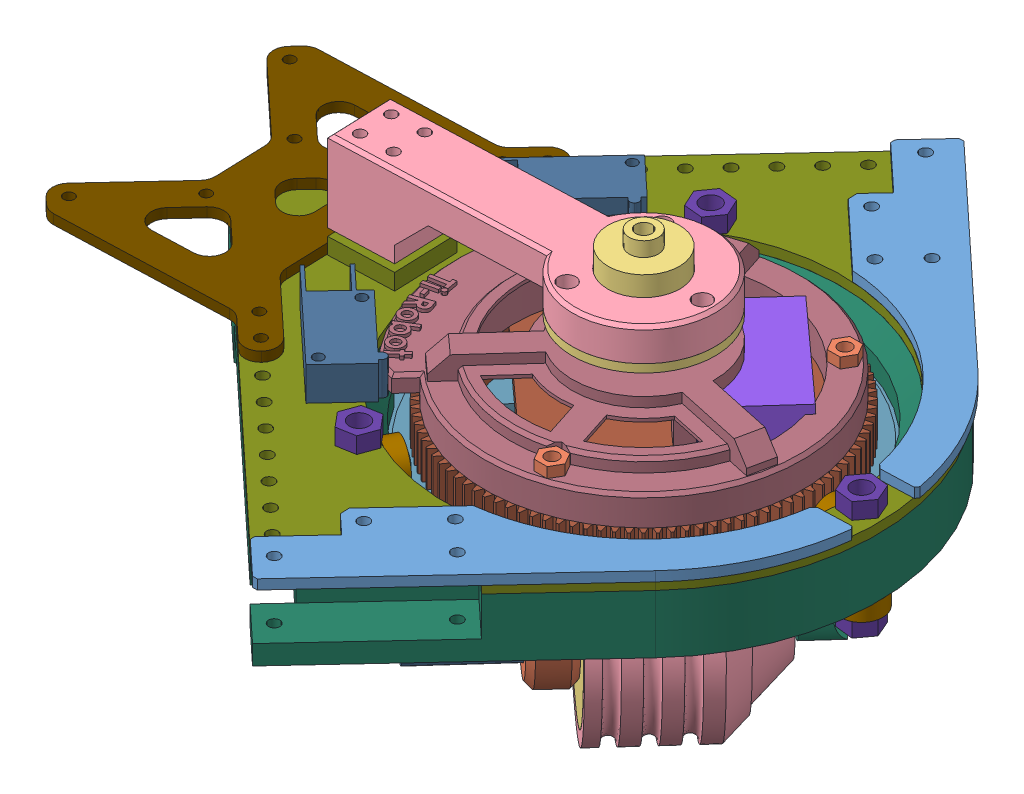
SolidWorks assembly swerve_unit, configuration ﾃﾞﾌｫﾙﾄ. Lengths in mm.
Overall size (282.67 132.43 227.55).
39 component instances, 23 part files, 96 mates.
Components (placement in the parent):
- M3508^swerve_unit-1: M3508^swerve_unit [ﾃﾞﾌｫﾙﾄ] at (107.8783 -47.57 102.4913) x (0 1 0) z (0.742238 0 0.670137) size (42 98.4 42) (virtual)
- motor_base^swerve_unit-1: motor_base^swerve_unit [ﾃﾞﾌｫﾙﾄ] at (107.8783 -47.57 102.4913) x (0 -1 0) z (0.670137 0 -0.742238) size (52 54 43) (virtual)
- bear_1^swerve_unit-1: bear_1^swerve_unit [ﾃﾞﾌｫﾙﾄ] at (129.3399 -43.5484 159.5919) x (0.723464 0.223485 0.653187) z (0.670137 0 -0.742238) size (72 72 12) (virtual)
- wheel^swerve_unit-1: wheel^swerve_unit [ﾃﾞﾌｫﾙﾄ] at (110.8472 -47.57 105.1718) x (0 1 0) z (0.742238 0 0.670137) size (80 47 80) (virtual)
- bear_2^swerve_unit-1: bear_2^swerve_unit [ﾃﾞﾌｫﾙﾄ] at (126.6421 -47.57 81.7086) x (0.245083 0.943913 0.221276) z (0.670137 0 -0.742238) size (26 26 8) (virtual)
- bear_cover^swerve_unit-1: bear_cover^swerve_unit [ﾃﾞﾌｫﾙﾄ] at (126.6421 -47.57 81.7086) x (0 -1 0) z (0.670137 0 -0.742238) size (43 40 11) (virtual)
- M2006^swerve_unit-1: M2006^swerve_unit [ﾃﾞﾌｫﾙﾄ] at (24.7128 -18.57 114.7671) x (0.883116 0 0.469155) z (0 -1 0) size (24.4 24.4 60.8) (virtual)
- C620^swerve_unit-1: C620^swerve_unit [ﾃﾞﾌｫﾙﾄ] at (40.7118 -3.57 117.3762) x (0.670137 0 -0.742238) z (0 1 0) size (25.8 49.4 11.6) (virtual)
- bear_3^swerve_unit-5: bear_3^swerve_unit [ﾃﾞﾌｫﾙﾄ] at (64.7019 -27.57 57.0296) x (-0.998139 0 0.060972) z (0 1 0) size (13 13 5) (virtual)
- bear_3^swerve_unit-6: bear_3^swerve_unit [ﾃﾞﾌｫﾙﾄ] at (164.1261 -27.57 109.8486) x (-0.435507 0 0.900185) z (0 1 0) size (13 13 5) (virtual)
- LS^swerve_unit-2: LS^swerve_unit [ﾃﾞﾌｫﾙﾄ] at (50.8347 9.23 168.1143) x (-0.731598 0 -0.681736) z (0 -1 0) size (37.8 18.1 10.3) (virtual)
- bear_3^swerve_unit-7: bear_3^swerve_unit [ﾃﾞﾌｫﾙﾄ] at (67.3531 -9.07 61.2689) x (-0.432819 -0.859886 0.270672) z (0.530223 0 0.847858) size (13 13 5) (virtual)
- steer_gear_2^swerve_unit-2: steer_gear_2^swerve_unit [ﾃﾞﾌｫﾙﾄ] at (187.3107 -27.57 157.2026) x (-0.951474 0 0.307728) z (-0.307728 0 -0.951474) size (101.97 11 101.97) (virtual)
- steer_gear_1^swerve_unit-2: steer_gear_1^swerve_unit [ﾃﾞﾌｫﾙﾄ] at (-26.2181 -27.57 -51.6068) x (0.883116 0 0.469155) z (-0.469155 0 0.883116) size (52 10 52.13) (virtual)
- striker^swerve_unit-4: striker^swerve_unit [ﾃﾞﾌｫﾙﾄ] at (99.1665 -3.57 112.1404) x (0.742238 0 0.670137) z (0 1 0) size (106.95 106.83 16) (virtual)
- steer_base^swerve_unit-5: steer_base^swerve_unit [ﾃﾞﾌｫﾙﾄ] at (99.1665 -22.57 112.1404) x (0.670137 0 -0.742238) z (0 1 0) size (120 120 13) (virtual)
- base^swerve_unit-2: base^swerve_unit [ﾃﾞﾌｫﾙﾄ] at (99.1665 -14.07 112.1404) x (0.731598 0 0.681736) z (0 1 0) size (160 160 19.28) (virtual)
- bear_3^swerve_unit-8: bear_3^swerve_unit [ﾃﾞﾌｫﾙﾄ] at (154.1323 -9.07 110.2012) x (0.032581 0.382218 0.923498) z (0.999378 0 -0.035258) size (13 13 5) (virtual)
- bear_3^swerve_unit-9: bear_3^swerve_unit [ﾃﾞﾌｫﾙﾄ] at (73.363 -9.07 160.7117) x (-0.532711 -0.797577 -0.283002) z (-0.469155 0 0.883116) size (13 13 5) (virtual)
- bear_3^swerve_unit-11: bear_3^swerve_unit [ﾃﾞﾌｫﾙﾄ] at (68.6714 -27.57 169.5429) x (-0.435507 0 0.900185) z (0 1 0) size (13 13 5) (virtual)
- base_cover^swerve_unit-1: base_cover^swerve_unit [ﾃﾞﾌｫﾙﾄ] at (99.1665 -4.07 112.1404) x (0.731598 0 0.681736) z (0 1 0) size (160 160 8) (virtual)
- LS^swerve_unit-3: LS^swerve_unit [ﾃﾞﾌｫﾙﾄ] at (47.0102 -1.07 59.7116) x (-0.681736 0 0.731598) z (0 1 0) size (37.8 18.1 10.3) (virtual)
- M6_nut^swerve_unit-2: M6_nut^swerve_unit [ﾃﾞﾌｫﾙﾄ] at (164.1261 -1.07 109.8486) x (0.398878 0 0.917004) z (0 1 0) size (11.55 10 5) (virtual)
- joint_frame^swerve_unit-1: joint_frame^swerve_unit [ﾃﾞﾌｫﾙﾄ] at origin size (162.53 3 162.53) (virtual)
  - Copy of Copy of Part48^joint_frame_swerve_unit-1: Copy of Copy of Part48^joint_frame_swerve_unit [ﾃﾞﾌｫﾙﾄ] at (86.927 -1.07 176.8816) x (-0.681736 0 0.731598) z (0 1 0) size (65 50 3) (hidden, virtual)
  - Copy of Copy of Part48^joint_frame_swerve_unit-2: Copy of Copy of Part48^joint_frame_swerve_unit [ﾃﾞﾌｫﾙﾄ] at (82.3949 1.93 48.4226) x (-0.731598 0 -0.681736) z (0 -1 0) size (65 50 3) (hidden, virtual)
  - Copy of alpt^joint_frame_swerve_unit-1: Copy of alpt^joint_frame_swerve_unit [ﾃﾞﾌｫﾙﾄ] at (86.927 1.93 176.8816) x (-0.681736 0 0.731598) z (0 1 0) size (115 115 3) (virtual)
- bamper^swerve_unit-1: bamper^swerve_unit [ﾃﾞﾌｫﾙﾄ] at (99.1665 -1.07 112.1404) x (0.731598 0 0.681736) z (0 1 0) size (26 131.43 3) (virtual)
- bamper^swerve_unit-2: bamper^swerve_unit [ﾃﾞﾌｫﾙﾄ] at (99.1665 1.93 112.1404) x (0.681736 0 -0.731598) z (0 -1 0) size (26 131.43 3) (virtual)
- M4_nut^swerve_unit-5: M4_nut^swerve_unit [ﾃﾞﾌｫﾙﾄ] at (56.1404 5.43 102.934) x (1 0 0) z (0 1 0) size (8.08 7 3.2) (virtual)
- M4_nut^swerve_unit-6: M4_nut^swerve_unit [ﾃﾞﾌｫﾙﾄ] at (128.6525 5.43 79.4819) x (1 0 0) z (0 1 0) size (8.08 7 3.2) (virtual)
- M4_nut^swerve_unit-7: M4_nut^swerve_unit [ﾃﾞﾌｫﾙﾄ] at (112.7065 5.43 154.0052) x (1 0 0) z (0 1 0) size (8.08 7 3.2) (virtual)
- slip_ring^swerve_unit-1: slip_ring^swerve_unit [ﾃﾞﾌｫﾙﾄ] at (99.1665 13.73 112.1404) x (0.999378 0 -0.035258) z (0 1 0) size (44 44 33) (virtual)
- slip_ring_base^swerve_unit-1: slip_ring_base^swerve_unit [ﾃﾞﾌｫﾙﾄ] at (99.1665 21.23 112.1404) x (0.999378 0 -0.035258) z (0 1 0) size (107 44 25) (virtual)
- M6_nut^swerve_unit-3: M6_nut^swerve_unit [ﾃﾞﾌｫﾙﾄ] at (68.6714 -1.07 169.5429) x (0.642883 0 0.765964) z (0 1 0) size (11.55 10 5) (virtual)
- M6_nut^swerve_unit-4: M6_nut^swerve_unit [ﾃﾞﾌｫﾙﾄ] at (164.1261 -32.57 109.8486) x (0.398878 0 0.917004) z (0 1 0) size (11.55 10 5) (virtual)
- M6_nut^swerve_unit-5: M6_nut^swerve_unit [ﾃﾞﾌｫﾙﾄ] at (68.6714 -32.57 169.5429) x (0.398878 0 0.917004) z (0 1 0) size (11.55 10 5) (virtual)
- M6_nut^swerve_unit-6: M6_nut^swerve_unit [ﾃﾞﾌｫﾙﾄ] at (64.7019 -32.57 57.0296) x (0.398878 0 0.917004) z (0 1 0) size (11.55 10 5) (virtual)
- M6_nut^swerve_unit-7: M6_nut^swerve_unit [ﾃﾞﾌｫﾙﾄ] at (64.7019 -1.07 57.0296) x (0.995843 0 0.091089) z (0 1 0) size (11.55 10 5) (virtual)
Mates (geometry in assembly coordinates):
- 相対固定5: in place: plane of ? through (-112.9944 -0.3949 73.4466) normal (0.707107 0 0.707107); plane of ? through (-19.7739 0 -19.7739) normal (0.707107 0 0.707107); moOrthogonalPlaneRef_w of ? through (-112.9944 -0.3949 73.4466) normal (0.707107 0 0.707107); plane of ? through (-19.7739 0 -19.7739) normal (0 1 0); plane of ? through (-112.9944 -0.3949 73.4466) normal (0.707107 0 0.707107); plane of ? through (-19.7739 0 -19.7739) normal (0.707107 0 -0.707107); plane of M3508^swerve_unit-1 through (107.8783 -47.57 102.4913) normal (0.670137 0 -0.742238); unknown of motor_base^swerve_unit-1
- 一致27: coincident aligned: plane of ?; plane of ?
- 一致28: coincident aligned: moOrthogonalPlaneRef_w of M3508^swerve_unit-1; plane of Part5^st3-1 through (107.8783 -47.57 102.4913) normal (-0.742238 0 -0.670137)
- 一致29: coincident anti-aligned: moOrthogonalPlaneRef_w of M3508^swerve_unit-1; plane of Part5^st3-1 through (107.8783 -47.57 102.4913) normal (0 -1 0)
- 同心円16: concentric anti-aligned: cylinder of Part5^st3-1 through (81.0728 -47.57 132.1808) axis (0.670137 0 -0.742238) radius 25; cylinder of Copy of Part1^st3-1 through (97.1561 -47.57 114.3671) axis (-0.670137 0 0.742238) radius 25
- 相対固定7: in place: plane of ? through (-22.8566 -14.0328 -4.7881) normal (0 -1 0); plane of ? through (0 -14.0328 0) normal (0 -1 0); plane of ? through (-22.8566 -14.0328 -4.7881) normal (0 -1 0); plane of ? through (0 -14.0328 0) normal (0 0 -1); plane of ? through (-22.8566 -14.0328 -4.7881) normal (0 -1 0); plane of ? through (0 -14.0328 0) normal (-1 0 0); plane of M3508^swerve_unit-1 through (110.8472 -47.57 105.1718) normal (0.742238 0 0.670137); unknown of wheel^swerve_unit-1
- 一致34: coincident aligned: plane of ?; plane of ?
- 一致35: coincident aligned: moOrthogonalPlaneRef_w of M3508^swerve_unit-1; plane of wheel^swerve_unit-1 through (110.8472 -47.57 105.1718) normal (-0.670137 0 0.742238)
- 一致36: coincident anti-aligned: moOrthogonalPlaneRef_w of M3508^swerve_unit-1; plane of wheel^swerve_unit-1 through (110.8472 -47.57 105.1718) normal (0 1 0)
- 一致37: coincident anti-aligned: plane of Copy of Part1^st3-1 through (97.1561 -47.57 114.3671) normal (0.670137 0 -0.742238); plane of wheel^swerve_unit-1 through (100.125 -47.57 117.0476) normal (-0.670137 0 0.742238)
- 同心円19: concentric anti-aligned: cylinder of M3508^swerve_unit-1 through (126.173 -47.57 82.2282) axis (-0.670137 0 0.742238) radius 5; cylinder of Part8^st3-1 through (121.281 -47.57 87.6465) axis (0.670137 0 -0.742238) radius 5
- 距離1: distance = 50 mm anti-aligned: plane of Part5^st3-1 through (87.7741 -47.57 124.7584) normal (0.670137 0 -0.742238); plane of Part9^st3-1 through (121.281 -47.57 87.6465) normal (-0.670137 0 0.742238)
- 同心円21: concentric aligned: cylinder of Part8^st3-1 through (121.281 -47.57 87.6465) axis (0.670137 0 -0.742238) radius 13; cylinder of Part9^st3-1 through (121.281 -47.57 87.6465) axis (0.670137 0 -0.742238) radius 13.15
- 一致52: coincident anti-aligned: plane of Part8^st3-1 through (126.6421 -47.57 81.7086) normal (0.670137 0 -0.742238); plane of Part9^st3-1 through (126.6421 -47.57 81.7086) normal (-0.670137 0 0.742238)
- 平行1: parallel aligned: plane of Part5^st3-1 through (107.8146 -47.57 142.8521) normal (0.742238 0 0.670137); plane of Part9^st3-1 through (142.0128 -22.57 91.5444) normal (0.742238 0 0.670137)
- 一致170: coincident aligned: plane of Copy of Copy of Copy of Copy (3) of Part3^st3-5 through (64.7019 -22.57 57.0296) normal (0 1 0); plane of Copy of Copy of Copy of Copy (3) of Part3^st3-6 through (164.1261 -22.57 109.8486) normal (0 1 0)
- 同心円103: concentric aligned: cylinder of Part30^st3-1 through (18.9886 -10.57 125.542) axis (0.469155 0 -0.883116) radius 1.5; cylinder of Copy of Assem1^st3-2 through (12.5203 -10.57 137.7178) axis (0.469155 0 -0.883116) radius 1.65
- 同心円106: concentric aligned: cylinder of Part30^st3-1 through (24.7128 -1.57 114.7671) axis (0 -1 0) radius 3; cylinder of Copy of Assem1^st3-2 through (24.7128 -4.569 114.7671) axis (0 -1 0) radius 3.1
- 同心円113: concentric anti-aligned: cylinder of Copy of Assem2^st3-2 through (99.1665 -54.5701 112.1404) axis (0 1 0) radius 40; cylinder of Part47^st3-4 through (99.1665 5.43 112.1404) axis (0 -1 0) radius 40
- 同心円114: concentric anti-aligned: cylinder of Copy of Assem2^st3-2 through (128.6525 -14.57 79.4819) axis (0 1 0) radius 2.15; cylinder of Part47^st3-4 through (128.6525 5.43 79.4819) axis (0 -1 0) radius 2.15
- 同心円115: concentric aligned: cylinder of Part9^st3-1 through (113.4981 -65.571 73.8833) axis (0 1 0) radius 2.25; cylinder of Part48^st3-5 through (113.4981 -25.57 73.8833) axis (0 1 0) radius 2.15
- 同心円116: concentric aligned: cylinder of Part9^st3-1 through (135.7652 -65.571 93.9874) axis (0 1 0) radius 2.25; cylinder of Part48^st3-5 through (135.7652 -25.57 93.9874) axis (0 1 0) radius 2.15
- 一致234: coincident anti-aligned: plane of Part9^st3-1 through (142.0128 -22.57 91.5444) normal (0 1 0); plane of Part48^st3-5 through (99.1665 -22.57 112.1404) normal (0 -1 0)
- 正接4: tangent anti-aligned: plane of Part48^st3-5 through (99.1665 -15.57 112.1404) normal (0 1 0); cylinder of Copy of Copy of Copy of Copy (3) of Part3^st3-9 through (71.0172 -9.07 165.1273) axis (0.469155 0 -0.883116) radius 6.5
- 正接5: tangent anti-aligned: plane of Part48^st3-5 through (99.1665 -15.57 112.1404) normal (0 1 0); cylinder of Copy of Copy of Copy of Copy (3) of Part3^st3-8 through (159.1292 -9.07 110.0249) axis (-0.999378 0 0.035258) radius 6.5
- 正接6: tangent anti-aligned: cylinder of Part48^st3-5 through (99.1665 -14.57 112.1404) axis (0 -1 0) radius 55; plane of Copy of Copy of Copy of Copy (3) of Part3^st3-8 through (154.1323 -9.07 110.2012) normal (-0.999378 0 0.035258)
- 正接7: tangent anti-aligned: cylinder of Part48^st3-5 through (99.1665 -14.57 112.1404) axis (0 -1 0) radius 55; plane of Copy of Copy of Copy of Copy (3) of Part3^st3-9 through (73.363 -9.07 160.7117) normal (0.469155 0 -0.883116)
- 正接9: tangent anti-aligned: cylinder of Copy of Copy of Copy of Copy (3) of Part3^st3-7 through (70.0042 -9.07 65.5082) axis (-0.530223 0 -0.847858) radius 6.5; plane of Part48^st3-5 through (99.1665 -15.57 112.1404) normal (0 1 0)
- 同心円123: concentric anti-aligned: cylinder of Copy of Copy of Copy of Copy (3) of Part3^st3-6 through (164.1261 -22.57 109.8486) axis (0 -1 0) radius 3; cylinder of Part49^st3-2 through (164.1261 -22.07 109.8486) axis (0 1 0) radius 3.15
- 一致246: coincident anti-aligned: plane of Copy of Copy of Copy of Copy (3) of Part3^st3-6 through (164.1261 -22.57 109.8486) normal (0 1 0); plane of Part48^st3-5 through (99.1665 -22.57 112.1404) normal (0 -1 0)
- 同心円124: concentric anti-aligned: cylinder of Part49^st3-2 through (73.8321 -9.07 159.8286) axis (-0.469155 0 0.883116) radius 3; cylinder of Copy of Copy of Copy of Copy (3) of Part3^st3-9 through (71.0172 -9.07 165.1273) axis (0.469155 0 -0.883116) radius 3
- 同心円125: concentric anti-aligned: cylinder of Part49^st3-2 through (153.1329 -9.07 110.2364) axis (0.999378 0 -0.035258) radius 3; cylinder of Copy of Copy of Copy of Copy (3) of Part3^st3-8 through (159.1292 -9.07 110.0249) axis (-0.999378 0 0.035258) radius 3
- 正接11: tangent anti-aligned: plane of Copy of Copy of Copy of Copy (3) of Part3^st3-7 through (70.0042 -9.07 65.5082) normal (0.530223 0 0.847858); cylinder of Part48^st3-5 through (99.1665 -14.57 112.1404) axis (0 -1 0) radius 55
- 同心円126: concentric aligned: cylinder of Copy of Copy of Copy of Copy (3) of Part3^st3-7 through (70.0042 -9.07 65.5082) axis (-0.530223 0 -0.847858) radius 3; cylinder of Part49^st3-2 through (70.5344 -9.07 66.356) axis (-0.530223 0 -0.847858) radius 3
- 一致247: coincident anti-aligned: plane of Copy of Copy of Copy of Copy (3) of Part3^st3-7 through (67.3531 -9.07 61.2689) normal (-0.530223 0 -0.847858); plane of Part49^st3-2 through (67.3531 -14.07 61.2689) normal (0.530223 0 0.847858)
- 一致248: coincident anti-aligned: plane of Part49^st3-2 through (159.1292 -14.07 110.0249) normal (-0.999378 0 0.035258); plane of Copy of Copy of Copy of Copy (3) of Part3^st3-8 through (159.1292 -9.07 110.0249) normal (0.999378 0 -0.035258)
- 一致249: coincident anti-aligned: plane of Part48^st3-5 through (99.1665 -22.57 112.1404) normal (0 -1 0); plane of Copy of Copy of Copy of Copy (3) of Part3^st3-11 through (68.6714 -22.57 169.5429) normal (0 1 0)
- 同心円127: concentric anti-aligned: cylinder of Part49^st3-2 through (68.6714 -22.07 169.5429) axis (0 1 0) radius 3.15; cylinder of Copy of Copy of Copy of Copy (3) of Part3^st3-11 through (68.6714 -22.57 169.5429) axis (0 -1 0) radius 3
- 一致250: coincident anti-aligned: plane of Copy of Copy of Copy of Copy (3) of Part3^st3-5 through (64.7019 -22.57 57.0296) normal (0 1 0); plane of Part48^st3-5 through (99.1665 -22.57 112.1404) normal (0 -1 0)
- 同心円128: concentric anti-aligned: cylinder of Copy of Copy of Copy of Copy (3) of Part3^st3-5 through (64.7019 -22.57 57.0296) axis (0 -1 0) radius 3; cylinder of Part49^st3-2 through (64.7019 -22.07 57.0296) axis (0 1 0) radius 3.15
- 同心円129: concentric aligned: circle of Copy of Assem2^st3-2; unknown of Part48^st3-5
- 一致251: coincident anti-aligned: plane of Copy of Assem2^st3-2 through (99.1665 -14.57 112.1404) normal (0 -1 0); plane of Part48^st3-5 through (99.1665 -14.57 112.1404) normal (0 1 0)
- 一致252: coincident anti-aligned: plane of Copy of Assem2^st3-2 through (83.3147 -4.57 94.8022) normal (0 -1 0); plane of Copy of Assem1^st3-2 through (24.7128 -4.57 114.7671) normal (0 1 0)
- 同心円130: concentric aligned: cylinder of Part30^st3-1 through (24.7128 -62.37 114.7671) axis (0 1 0) radius 12.2; cylinder of Part49^st3-2 through (24.7128 -22.07 114.7671) axis (0 1 0) radius 12.25
- 相対固定9: in place: plane of base^swerve_unit-2 through (99.1665 -4.07 112.1404) normal (0 1 0); plane of ? through (0 -4.07 0) normal (0 1 0); plane of base^swerve_unit-2 through (99.1665 -4.07 112.1404) normal (0 1 0); plane of ? through (0 -4.07 0) normal (0 0 -1); plane of base^swerve_unit-2 through (99.1665 -4.07 112.1404) normal (0 1 0); plane of ? through (0 -4.07 0) normal (1 0 0); plane of base^swerve_unit-2 through (99.1665 -4.07 112.1404) normal (0 1 0); unknown of base_cover^swerve_unit-1
- 一致253: coincident aligned: plane of ?; plane of ?
- 一致254: coincident aligned: moOrthogonalPlaneRef_w of Part49^st3-2 through (99.1665 -4.07 112.1404) normal (0.681736 0 -0.731598); plane of Part50^st3-1 through (99.1665 -4.07 112.1404) normal (0.681736 0 -0.731598)
- 一致255: coincident anti-aligned: moOrthogonalPlaneRef_w of Part49^st3-2 through (99.1665 -4.07 112.1404) normal (-0.731598 0 -0.681736); plane of Part50^st3-1 through (99.1665 -4.07 112.1404) normal (0.731598 0 0.681736)
- 一致257: coincident anti-aligned: plane of Part44^st3-2 through (50.8347 -1.07 168.1143) normal (0 -1 0); plane of Part50^st3-1 through (99.1665 -1.07 112.1404) normal (0 1 0)
- 平行2: parallel aligned: plane of Part44^st3-2 through (50.8347 -1.07 168.1143) normal (-0.681736 0 0.731598); plane of Part49^st3-2 through (91.8488 -4.07 225.606) normal (-0.681736 0 0.731598)
- 同心円131: concentric aligned: cylinder of Part44^st3-2 through (41.4754 -1.07 141.487) axis (0 1 0) radius 1.55; cylinder of Part50^st3-1 through (41.4754 -21.07 141.487) axis (0 1 0) radius 1.7
- 一致261: coincident anti-aligned: plane of Part50^st3-1 through (99.1665 -1.07 112.1404) normal (0 1 0); plane of Part44^st3-3 through (47.0102 -1.07 59.7116) normal (0 -1 0)
- 同心円132: concentric anti-aligned: cylinder of Part50^st3-1 through (47.1498 -21.07 63.6689) axis (0 1 0) radius 1.7; cylinder of Part44^st3-3 through (47.1498 9.23 63.6689) axis (0 -1 0) radius 1.55
- 同心円133: concentric anti-aligned: cylinder of Part50^st3-1 through (39.5508 -21.07 86.9323) axis (0 1 0) radius 1.7; cylinder of Part44^st3-3 through (39.5508 9.23 86.9323) axis (0 -1 0) radius 1.55
- 一致263: coincident anti-aligned: plane of Part50^st3-1 through (99.1665 -1.07 112.1404) normal (0 1 0); plane of Copy (2) of Part36^st3-2 through (164.1261 -1.07 109.8486) normal (0 -1 0)
- 同心円135: concentric aligned: cylinder of Part50^st3-1 through (164.1261 -1.07 109.8486) axis (0 -1 0) radius 3.15; cylinder of Copy (2) of Part36^st3-2 through (164.1261 3.93 109.8486) axis (0 -1 0) radius 3
- 同心円140: concentric anti-aligned: cylinder of Part47^st3-4 through (56.1404 5.43 102.934) axis (0 -1 0) radius 2.15; cylinder of Part48^st3-5 through (56.1404 -27.571 102.934) axis (0 1 0) radius 2.15
- 相対固定10: in place: plane of base_cover^swerve_unit-1 through (99.1665 -1.07 112.1404) normal (0 1 0); plane of ? through (0 -1.07 0) normal (0 1 0); plane of base_cover^swerve_unit-1 through (99.1665 -1.07 112.1404) normal (0 1 0); plane of ? through (0 -1.07 0) normal (0 0 -1); plane of base_cover^swerve_unit-1 through (99.1665 -1.07 112.1404) normal (0 1 0); plane of ? through (0 -1.07 0) normal (1 0 0); plane of base_cover^swerve_unit-1 through (99.1665 -1.07 112.1404) normal (0 1 0); unknown of bamper^swerve_unit-1
- 一致272: coincident aligned: plane of ?; plane of ?
- 一致273: coincident aligned: moOrthogonalPlaneRef_w of Part50^st3-1 through (99.1665 -1.07 112.1404) normal (0.681736 0 -0.731598); plane of Part51^st3-1 through (99.1665 -1.07 112.1404) normal (0.681736 0 -0.731598)
- 一致274: coincident anti-aligned: moOrthogonalPlaneRef_w of Part50^st3-1 through (99.1665 -1.07 112.1404) normal (-0.731598 0 -0.681736); plane of Part51^st3-1 through (99.1665 -1.07 112.1404) normal (0.731598 0 0.681736)
- 一致275: coincident anti-aligned: plane of Part50^st3-1 through (99.1665 -1.07 112.1404) normal (0 1 0); plane of Part51^st3-2 through (99.1665 -1.07 112.1404) normal (0 -1 0)
- 同心円145: concentric aligned: cylinder of Part49^st3-2 through (82.4158 -22.071 8.3682) axis (0 1 0) radius 1.75; cylinder of Part51^st3-2 through (82.4158 -1.07 8.3682) axis (0 1 0) radius 1.75
- 同心円146: concentric aligned: cylinder of Part49^st3-2 through (111.6797 -22.071 35.6376) axis (0 1 0) radius 1.75; cylinder of Part51^st3-2 through (111.6797 -1.07 35.6376) axis (0 1 0) radius 1.75
- 同心円147: concentric aligned: cylinder of Part30^st3-1 through (19.6757 -23.57 106.7124) axis (0 1 0) radius 1.5; cylinder of Part49^st3-2 through (19.6757 -22.07 106.7124) axis (0 1 0) radius 1.7
- 一致286: coincident anti-aligned: plane of Part47^st3-4 through (99.1665 5.43 112.1404) normal (0 1 0); plane of Part46^st3-5 through (56.1404 5.43 102.934) normal (0 -1 0)
- 同心円155: concentric aligned: cylinder of Part47^st3-4 through (56.1404 5.43 102.934) axis (0 -1 0) radius 2.15; cylinder of Part46^st3-5 through (56.1404 8.63 102.934) axis (0 -1 0) radius 2
- 一致287: coincident anti-aligned: plane of Part47^st3-4 through (99.1665 5.43 112.1404) normal (0 1 0); plane of Part46^st3-6 through (128.6525 5.43 79.4819) normal (0 -1 0)
- 同心円156: concentric aligned: cylinder of Part47^st3-4 through (128.6525 5.43 79.4819) axis (0 -1 0) radius 2.15; cylinder of Part46^st3-6 through (128.6525 8.63 79.4819) axis (0 -1 0) radius 2
- 一致288: coincident anti-aligned: plane of Part47^st3-4 through (99.1665 5.43 112.1404) normal (0 1 0); plane of Part46^st3-7 through (112.7065 5.43 154.0052) normal (0 -1 0)
- 同心円157: concentric aligned: cylinder of Part47^st3-4 through (112.7065 5.43 154.0052) axis (0 -1 0) radius 2.15; cylinder of Part46^st3-7 through (112.7065 8.63 154.0052) axis (0 -1 0) radius 2
- 同心円158: concentric anti-aligned: cylinder of Copy of Assem2^st3-2 through (99.1665 -54.5701 112.1404) axis (0 1 0) radius 40; cylinder of Part53^st3-1 through (99.1665 37.23 112.1404) axis (0 -1 0) radius 11
- 相対固定12: in place: plane of ? through (99.1665 49.0644 112.1404) normal (0 1 0); plane of ? through (0 49.0644 0) normal (0 1 0); plane of ? through (99.1665 49.0644 112.1404) normal (0 1 0); plane of ? through (0 49.0644 0) normal (0 0 -1); plane of ? through (99.1665 49.0644 112.1404) normal (0 1 0); plane of ? through (0 49.0644 0) normal (1 0 0); plane of slip_ring^swerve_unit-1 through (99.1665 21.23 112.1404) normal (0 1 0); unknown of slip_ring_base^swerve_unit-1
- 一致296: coincident aligned: plane of ?; plane of ?
- 一致297: coincident aligned: moOrthogonalPlaneRef_w of Part53^st3-1; plane of Copy of Part54^st3-1 through (99.1665 21.23 112.1404) normal (-0.035258 0 -0.999378)
- 一致298: coincident anti-aligned: unknown of Part53^st3-1; plane of Copy of Part54^st3-1 through (99.1665 21.23 112.1404) normal (0.999378 0 -0.035258)
- 平行5: parallel aligned: plane of Part49^st3-2 through (-17.891 -4.07 123.3456) normal (-0.999378 0 0.035258); plane of Copy of Part54^st3-1 through (14.2193 21.23 115.1373) normal (-0.999378 0 0.035258)
- 一致300: coincident anti-aligned: plane of Copy of Assem2^st3-2 through (83.3147 -3.57 94.8022) normal (0 1 0); plane of Part47^st3-4 through (99.1665 -3.57 112.1404) normal (0 -1 0)
- 一致303: coincident anti-aligned: plane of Part31^st3-1 through (141.9348 8.03 101.6287) normal (0.670137 0 -0.742238); plane of Part47^st3-4 through (123.6016 -1.07 85.0763) normal (-0.670137 0 0.742238)
- 一致304: coincident anti-aligned: plane of Part31^st3-1 through (141.9348 8.03 101.6287) normal (0.742238 0 0.670137); plane of Part47^st3-4 through (117.4997 -1.07 128.6927) normal (-0.742238 0 -0.670137)
- 距離2: distance = 2.3 mm anti-aligned: plane of Part50^st3-1 through (99.1665 3.93 112.1404) normal (0 1 0); plane of Copy of Part54^st3-1 through (99.1665 6.23 112.1404) normal (0 -1 0)
- 一致306: coincident aligned: plane of Part31^st3-1 through (40.7118 -3.57 117.3762) normal (0 -1 0); plane of Part47^st3-4 through (99.1665 -3.57 112.1404) normal (0 -1 0)
- 一致307: coincident anti-aligned: plane of Part50^st3-1 through (99.1665 -1.07 112.1404) normal (0 1 0); plane of Assem1^st3-1/Copy of Copy of Part48^Assem1_st3-1 through (86.927 -1.07 176.8816) normal (0 -1 0)
- 同心円159: concentric anti-aligned: cylinder of Part50^st3-1 through (19.3552 -4.071 76.041) axis (0 1 0) radius 1.75; cylinder of Assem1^st3-1/Copy of Copy of Part48^Assem1_st3-1 through (19.3552 1.93 76.041) axis (0 -1 0) radius 1.65
- 一致308: coincident anti-aligned: plane of Part50^st3-1 through (99.1665 -1.07 112.1404) normal (0 1 0); plane of Assem1^st3-1/Copy of Copy of Part48^Assem1_st3-2 through (82.3949 -1.07 48.4226) normal (0 -1 0)
- 同心円162: concentric aligned: cylinder of Part50^st3-1 through (22.0976 -4.071 153.7744) axis (0 1 0) radius 1.75; cylinder of Assem1^st3-1/Copy of Copy of Part48^Assem1_st3-2 through (22.0976 -1.07 153.7744) axis (0 1 0) radius 1.65
- 同心円163: concentric aligned: cylinder of base_cover^st3-1 through (68.6714 -1.07 169.5429) axis (0 -1 0) radius 3.15; cylinder of M6_nut^st3-3 through (68.6714 3.93 169.5429) axis (0 -1 0) radius 3
- 同心円164: concentric aligned: cylinder of base_cover^st3-1 through (64.7019 -1.07 57.0296) axis (0 -1 0) radius 3.15; cylinder of M6_nut^st3-7 through (64.7019 3.93 57.0296) axis (0 -1 0) radius 3
- 一致309: coincident anti-aligned: plane of base_cover^st3-1 through (99.1665 -1.07 112.1404) normal (0 1 0); plane of M6_nut^st3-7 through (64.7019 -1.07 57.0296) normal (0 -1 0)
- 一致310: coincident anti-aligned: plane of base_cover^st3-1 through (99.1665 -1.07 112.1404) normal (0 1 0); plane of M6_nut^st3-3 through (68.6714 -1.07 169.5429) normal (0 -1 0)
- 一致311: coincident anti-aligned: plane of bear_3^st3-11 through (68.6714 -27.57 169.5429) normal (0 -1 0); plane of M6_nut^st3-5 through (68.6714 -27.57 169.5429) normal (0 1 0)
- 一致312: coincident anti-aligned: plane of bear_3^st3-5 through (64.7019 -27.57 57.0296) normal (0 -1 0); plane of M6_nut^st3-6 through (64.7019 -27.57 57.0296) normal (0 1 0)
- 一致313: coincident anti-aligned: plane of bear_3^st3-6 through (164.1261 -27.57 109.8486) normal (0 -1 0); plane of M6_nut^st3-4 through (164.1261 -27.57 109.8486) normal (0 1 0)
- 同心円165: concentric aligned: cylinder of bear_3^st3-6 through (164.1261 -22.57 109.8486) axis (0 -1 0) radius 3; cylinder of M6_nut^st3-4 through (164.1261 -27.57 109.8486) axis (0 -1 0) radius 3
- 同心円166: concentric aligned: cylinder of bear_3^st3-5 through (64.7019 -22.57 57.0296) axis (0 -1 0) radius 3; cylinder of M6_nut^st3-6 through (64.7019 -27.57 57.0296) axis (0 -1 0) radius 3
- 同心円167: concentric aligned: cylinder of bear_3^st3-11 through (68.6714 -22.57 169.5429) axis (0 -1 0) radius 3; cylinder of M6_nut^st3-5 through (68.6714 -27.57 169.5429) axis (0 -1 0) radius 3
